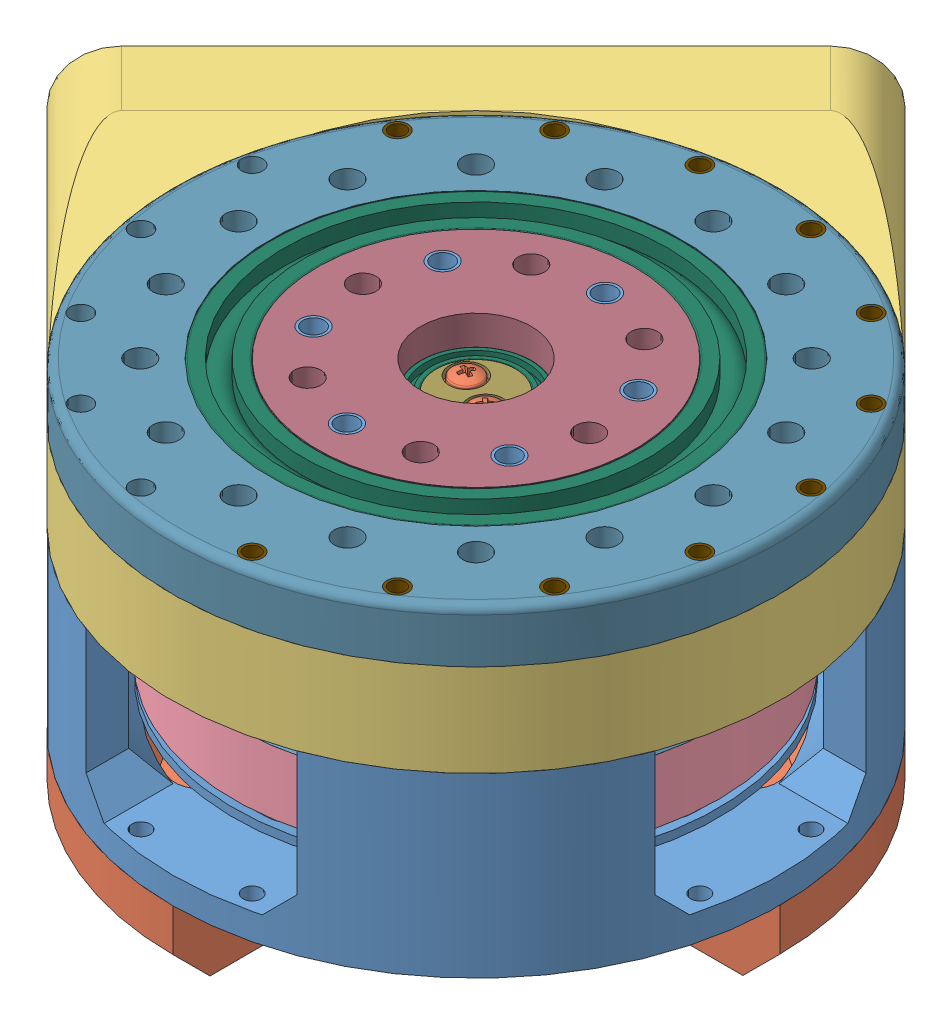
SolidWorks assembly Cycloidal_v2, configuration Default. Lengths in mm. (continued)
Components (placement in the parent): (continued)
- hex nut style 1 gradeab_iso-1: hex nut style 1 gradeab_iso [ISO - 4032 - M3 - W - N] at (47.267 33.7573 119.5643) x (1 0 0) z (0 -1 0) size (5.5 6.35 2.4)
- Cycloidal_Discs_8308-1: Cycloidal_Discs_8308 [Default] at (41.9439 42.227 18.4807) x (0.879085 0 0.476665) z (-0.476665 0 0.879085) size (79.25 5 79.73)
  - Cycloidal_Discs-1: Cycloidal_Discs [Default] at (38.3081 39.5303 58.0959) size (79.25 5 79.73)
  - radial ball bearing_68_iso-1: radial ball bearing_68_iso [ISO 15 RBB - 274 - 14,SI,NC,14_68] at (18.3896 43.2803 46.5959) x (0 1 0) z (0 0 1) size (2.5 7 7)
  - radial ball bearing_68_iso-2: radial ball bearing_68_iso [ISO 15 RBB - 274 - 14,SI,NC,14_68] at (38.3081 43.2803 81.0959) x (0 1 0) z (0 0 1) size (2.5 7 7)
  - radial ball bearing_68_iso-3: radial ball bearing_68_iso [ISO 15 RBB - 274 - 14,SI,NC,14_68] at (18.3896 43.2803 69.5959) x (0 1 0) z (0 0 1) size (2.5 7 7)
  - radial ball bearing_68_iso-4: radial ball bearing_68_iso [ISO 15 RBB - 274 - 14,SI,NC,14_68] at (38.3081 43.2803 35.0959) x (0 1 0) z (0 0 1) size (2.5 7 7)
  - radial ball bearing_68_iso-5: radial ball bearing_68_iso [ISO 15 RBB - 274 - 14,SI,NC,14_68] at (58.2267 43.2803 69.5959) x (0 1 0) z (0 0 1) size (2.5 7 7)
  - radial ball bearing_68_iso-6: radial ball bearing_68_iso [ISO 15 RBB - 274 - 14,SI,NC,14_68] at (58.2267 43.2803 46.5959) x (0 1 0) z (0 0 1) size (2.5 7 7)
- Cycloidal_Discs_8308-2: Cycloidal_Discs_8308 [Default] at (110.2095 37.227 62.2693) x (-0.1644 0 0.986394) z (-0.986394 0 -0.1644) size (79.25 5 79.73)
  - Cycloidal_Discs-1: Cycloidal_Discs [Default] at (38.3081 39.5303 58.0959) size (79.25 5 79.73)
  - radial ball bearing_68_iso-1: radial ball bearing_68_iso [ISO 15 RBB - 274 - 14,SI,NC,14_68] at (18.3896 43.2803 46.5959) x (0 1 0) z (0 0 1) size (2.5 7 7)
  - radial ball bearing_68_iso-2: radial ball bearing_68_iso [ISO 15 RBB - 274 - 14,SI,NC,14_68] at (38.3081 43.2803 81.0959) x (0 1 0) z (0 0 1) size (2.5 7 7)
  - radial ball bearing_68_iso-3: radial ball bearing_68_iso [ISO 15 RBB - 274 - 14,SI,NC,14_68] at (18.3896 43.2803 69.5959) x (0 1 0) z (0 0 1) size (2.5 7 7)
  - radial ball bearing_68_iso-4: radial ball bearing_68_iso [ISO 15 RBB - 274 - 14,SI,NC,14_68] at (38.3081 43.2803 35.0959) x (0 1 0) z (0 0 1) size (2.5 7 7)
  - radial ball bearing_68_iso-5: radial ball bearing_68_iso [ISO 15 RBB - 274 - 14,SI,NC,14_68] at (58.2267 43.2803 69.5959) x (0 1 0) z (0 0 1) size (2.5 7 7)
  - radial ball bearing_68_iso-6: radial ball bearing_68_iso [ISO 15 RBB - 274 - 14,SI,NC,14_68] at (58.2267 43.2803 46.5959) x (0 1 0) z (0 0 1) size (2.5 7 7)
- m6-1: m6 [Default] at (24.3171 92.633 87.6415) x (0 0 -1) z (-1 0 0) size (6 16 6)
- Motor_Cover_v2-2: Motor_Cover_v2 [Default] at (47.267 36.1573 89.1587) x (-1 0 0) z (0 0 -1) size (115 33.6 115)
- driver_cover-1: driver_cover [Default] at (47.267 36.1573 89.1587) x (-0.70834 0 -0.705872) z (-0.705872 0 0.70834) size (81.32 15 115)
- Base_plate_2 _new-1: Base_plate_2 _new [Default] at (47.267 69.6573 89.1587) x (-0.707107 0 0.707107) z (-0.707107 0 -0.707107) size (115 87.5 130)
Mates (geometry in assembly coordinates):
- Coincident1: coincident anti-aligned: plane of motor-X83008S.stp-1/outrunner.stp-1 through (62.4642 69.7573 58.1862) normal (0 1 0); plane of Base_Plate-1 through (47.267 69.7573 89.1587) normal (0 -1 0)
- Concentric1: concentric anti-aligned: line of motor-X83008S.stp-1/outrunner.stp-1 through (54.0947 64.2573 75.2435) axis (0 1 0); cylinder of Base_Plate-1 through (54.0947 76.7573 75.2435) axis (0 -1 0) radius 1.5
- Concentric2: concentric anti-aligned: cylinder of motor-X83008S.stp-1/shaft.stp-1 through (47.267 69.7573 89.1587) axis (0 1 0) radius 1.5; line of Base_Plate-1 through (47.267 76.7573 89.1587) axis (0 -1 0)
- Coincident2: coincident anti-aligned: plane of Base_Plate-1 through (47.267 76.7573 89.1587) normal (0 1 0); plane of Eccentric_Shaft-1/Eccentric_Shaft_bot-1 through (46.6062 76.7573 90.5053) normal (0 -1 0)
- Concentric75: concentric anti-aligned: cylinder of Output_Shaft-1 through (47.267 97.2573 89.1587) axis (0 -1 0) radius 30; cylinder of radial ball bearing_68_iso-39 through (47.267 71.6198 89.1587) axis (0 1 0) radius 30
- Concentric76: concentric anti-aligned: cylinder of Cover-1 through (47.267 97.2573 89.1587) axis (0 -1 0) radius 39; cylinder of radial ball bearing_68_iso-39 through (47.267 71.6198 89.1587) axis (0 1 0) radius 39
- Coincident104: coincident aligned: plane of Cover-1 through (47.267 97.2573 89.1587) normal (0 1 0); plane of radial ball bearing_68_iso-39 through (8.567 97.2573 89.1587) normal (0 1 0)
- Coincident105: coincident aligned: plane of Output_Shaft-1 through (47.267 97.2573 89.1587) normal (0 1 0); plane of Cover-1 through (47.267 97.2573 89.1587) normal (0 1 0)
- Concentric78: concentric anti-aligned: cylinder of Base_Plate-1 through (47.267 76.7573 89.1587) axis (0 -1 0) radius 20; cylinder of radial ball bearing_68_iso-40 through (47.267 52.6198 89.1587) axis (0 1 0) radius 20
- Concentric84: concentric aligned: cylinder of Cover-1 through (15.4472 87.2573 57.3389) axis (0 1 0) radius 2.5; cylinder of m13_bearing-1/m6-1 through (15.4472 86.8573 57.3389) axis (0 1 0) radius 2
- Concentric85: concentric aligned: cylinder of Cover-1 through (47.267 87.2573 134.1587) axis (0 1 0) radius 2.5; cylinder of m13_bearing-11/m6-1 through (47.267 86.8573 134.1587) axis (0 1 0) radius 2
- Concentric86: concentric aligned: cylinder of Cover-1 through (64.4877 87.2573 130.7332) axis (0 1 0) radius 2.5; cylinder of m13_bearing-2/m6-1 through (64.4877 86.8573 130.7332) axis (0 1 0) radius 2
- Concentric87: concentric aligned: cylinder of Cover-1 through (79.0868 87.2573 120.9785) axis (0 1 0) radius 2.5; cylinder of m13_bearing-12/m6-1 through (79.0868 86.8573 120.9785) axis (0 1 0) radius 2
- Concentric88: concentric aligned: cylinder of Cover-1 through (88.8416 87.2573 106.3794) axis (0 1 0) radius 2.5; cylinder of m13_bearing-5/m6-1 through (88.8416 86.8573 106.3794) axis (0 1 0) radius 2
- Concentric89: concentric aligned: cylinder of Cover-1 through (92.267 87.2573 89.1587) axis (0 1 0) radius 2.5; cylinder of m13_bearing-4/m6-1 through (92.267 86.8573 89.1587) axis (0 1 0) radius 2
- Concentric90: concentric aligned: cylinder of Cover-1 through (30.0462 87.2573 47.5841) axis (0 1 0) radius 2.5; cylinder of m13_bearing-6/m6-1 through (30.0462 86.8573 47.5841) axis (0 1 0) radius 2
- Concentric91: concentric aligned: cylinder of Cover-1 through (47.267 87.2573 44.1587) axis (0 1 0) radius 2.5; cylinder of m13_bearing-3/m6-1 through (47.267 86.8573 44.1587) axis (0 1 0) radius 2
- Concentric92: concentric aligned: cylinder of Cover-1 through (64.4877 87.2573 47.5841) axis (0 1 0) radius 2.5; cylinder of m13_bearing-7/m6-1 through (64.4877 86.8573 47.5841) axis (0 1 0) radius 2
- Concentric93: concentric aligned: cylinder of Cover-1 through (79.0868 87.2573 57.3389) axis (0 1 0) radius 2.5; cylinder of m13_bearing-8/m6-1 through (79.0868 86.8573 57.3389) axis (0 1 0) radius 2
- Concentric94: concentric aligned: cylinder of Cover-1 through (88.8416 87.2573 71.9379) axis (0 1 0) radius 2.5; cylinder of m13_bearing-9/m6-1 through (88.8416 86.8573 71.9379) axis (0 1 0) radius 2
- Concentric118: concentric anti-aligned: cylinder of Output_Shaft-1 through (60.0558 97.2573 70.042) axis (0 -1 0) radius 2.5; cylinder of M4x6x5.5_brass_insert-1 through (60.0558 86.633 70.042) axis (0 1 0) radius 2
- Concentric1211: concentric aligned: cylinder of Cover-1 through (2.3676 97.2573 59.1579) axis (0 -1 0) radius 2; cylinder of M3x4x4.2_brass_insert-2 through (2.3676 92.3553 59.1579) axis (0 -1 0) radius 1.5
- Concentric1221: concentric aligned: cylinder of Cover-1 through (17.2662 97.2573 44.2593) axis (0 -1 0) radius 2; cylinder of M3x4x4.2_brass_insert-3 through (17.2662 92.3553 44.2593) axis (0 -1 0) radius 1.5
- Concentric1251: concentric aligned: cylinder of Cover-1 through (77.2678 97.2573 44.2593) axis (0 -1 0) radius 2; cylinder of M3x4x4.2_brass_insert-6 through (77.2678 92.3553 44.2593) axis (0 -1 0) radius 1.8
- Concentric1271: concentric anti-aligned: cylinder of Cover-1 through (100.2294 97.2573 78.6238) axis (0 -1 0) radius 2; cylinder of M3x4x4.2_brass_insert-8 through (100.2294 98.1594 78.6238) axis (0 1 0) radius 1.8
- Concentric1331: concentric aligned: cylinder of Cover-1 through (36.7321 97.2573 36.1963) axis (0 -1 0) radius 2; cylinder of M3x4x4.2_brass_insert-14 through (36.7321 92.3553 36.1963) axis (0 -1 0) radius 1.8
- Concentric1341: concentric anti-aligned: cylinder of Cover-1 through (57.8019 97.2573 36.1963) axis (0 -1 0) radius 2; cylinder of M3x4x4.2_brass_insert-15 through (57.8019 98.1594 36.1963) axis (0 1 0) radius 2
- Concentric1351: concentric aligned: cylinder of Cover-1 through (92.1663 97.2573 59.1579) axis (0 -1 0) radius 2; cylinder of M3x4x4.2_brass_insert-16 through (92.1663 92.3553 59.1579) axis (0 -1 0) radius 2
- Concentric1361: concentric aligned: cylinder of Cover-1 through (100.2294 97.2573 99.6935) axis (0 -1 0) radius 2; cylinder of M3x4x4.2_brass_insert-17 through (100.2294 92.3553 99.6935) axis (0 -1 0) radius 2
- Concentric1381: concentric aligned: cylinder of Cover-1 through (92.1663 97.2573 119.1595) axis (0 -1 0) radius 2; cylinder of M3x4x4.2_brass_insert-19 through (92.1663 92.3553 119.1595) axis (0 -1 0) radius 2
- Concentric1391: concentric aligned: cylinder of Cover-1 through (77.2678 97.2573 134.058) axis (0 -1 0) radius 2; cylinder of M3x4x4.2_brass_insert-20 through (77.2678 92.3553 134.058) axis (0 -1 0) radius 1.5
- Concentric1401: concentric aligned: cylinder of Cover-1 through (57.8019 97.2573 142.1211) axis (0 -1 0) radius 2; cylinder of M3x4x4.2_brass_insert-21 through (57.8019 92.3553 142.1211) axis (0 -1 0) radius 1.5
- Concentric14021: concentric aligned: cylinder of Output_Shaft-1 through (57.4281 97.2573 109.7924) axis (0 -1 0) radius 2.5; cylinder of M4x6x5.5_brass_insert-4 through (57.4281 80.689 109.7924) axis (0 -1 0) radius 2.5
- Concentric14031: concentric aligned: cylinder of Output_Shaft-1 through (34.4782 97.2573 108.2753) axis (0 -1 0) radius 2.5; cylinder of M4x6x5.5_brass_insert-5 through (34.4782 80.689 108.2753) axis (0 -1 0) radius 2.5
- Concentric14041: concentric aligned: cylinder of Output_Shaft-1 through (24.3171 97.2573 87.6415) axis (0 -1 0) radius 2.5; cylinder of M4x6x5.5_brass_insert-6 through (24.3171 80.689 87.6415) axis (0 -1 0) radius 2.5
- Concentric14051: concentric aligned: cylinder of Output_Shaft-1 through (37.1059 97.2573 68.5249) axis (0 -1 0) radius 2.5; cylinder of M4x6x5.5_brass_insert-7 through (37.1059 80.689 68.5249) axis (0 -1 0) radius 2.5
- Concentric14061: concentric aligned: cylinder of Output_Shaft-1 through (67.9008 97.2573 78.9976) axis (0 -1 0) radius 2.5; cylinder of M4x6x5.5_brass_insert-8 through (67.9008 85.3133 78.9976) axis (0 -1 0) radius 2.5
- Concentric14071: concentric aligned: cylinder of Output_Shaft-1 through (48.7841 97.2573 66.2088) axis (0 -1 0) radius 2.5; cylinder of M4x6x5.5_brass_insert-9 through (48.7841 85.3133 66.2088) axis (0 -1 0) radius 2.5
- Concentric14081: concentric aligned: cylinder of Output_Shaft-1 through (28.1503 97.2573 76.3698) axis (0 -1 0) radius 2.5; cylinder of M4x6x5.5_brass_insert-10 through (28.1503 85.3133 76.3698) axis (0 -1 0) radius 2.5
- Concentric14091: concentric aligned: cylinder of Output_Shaft-1 through (26.6332 97.2573 99.3197) axis (0 -1 0) radius 2.5; cylinder of M4x6x5.5_brass_insert-11 through (26.6332 85.3133 99.3197) axis (0 -1 0) radius 2.5
- Concentric14111: concentric aligned: cylinder of Output_Shaft-1 through (45.7499 97.2573 112.1086) axis (0 -1 0) radius 2.5; cylinder of M4x6x5.5_brass_insert-13 through (45.7499 85.3133 112.1086) axis (0 -1 0) radius 2.5
- Concentric14121: concentric aligned: cylinder of Output_Shaft-1 through (66.3836 97.2573 101.9475) axis (0 -1 0) radius 2.5; cylinder of M4x6x5.5_brass_insert-14 through (66.3836 85.3133 101.9475) axis (0 -1 0) radius 2.5
- Concentric14131: concentric aligned: cylinder of Output_Shaft-1 through (70.2169 97.2573 90.6758) axis (0 -1 0) radius 2.5; cylinder of M4x6x5.5_brass_insert-15 through (70.2169 80.689 90.6758) axis (0 -1 0) radius 2.5
- Coincident1435: coincident aligned: plane of M4x6x5.5_brass_insert-1 through (58.1912 92.633 71.7074) normal (0 1 0); plane of M4x6x5.5_brass_insert-15 through (70.2169 92.633 90.6758) normal (0 1 0)
- Coincident1436: coincident aligned: plane of M4x6x5.5_brass_insert-1 through (58.1912 92.633 71.7074) normal (0 1 0); plane of M4x6x5.5_brass_insert-4 through (57.4281 92.633 109.7924) normal (0 1 0)
- Coincident1437: coincident aligned: plane of M4x6x5.5_brass_insert-1 through (58.1912 92.633 71.7074) normal (0 1 0); plane of M4x6x5.5_brass_insert-5 through (34.4782 92.633 108.2753) normal (0 1 0)
- Coincident1438: coincident aligned: plane of M4x6x5.5_brass_insert-1 through (58.1912 92.633 71.7074) normal (0 1 0); plane of M4x6x5.5_brass_insert-6 through (24.3171 92.633 87.6415) normal (0 1 0)
- Coincident1439: coincident aligned: plane of M4x6x5.5_brass_insert-1 through (58.1912 92.633 71.7074) normal (0 1 0); plane of M4x6x5.5_brass_insert-7 through (37.1059 92.633 68.5249) normal (0 1 0)
- Coincident1440: coincident aligned: plane of Output_Shaft-1 through (47.267 97.2573 89.1587) normal (0 1 0); plane of M4x6x5.5_brass_insert-9 through (48.7841 97.2573 66.2088) normal (0 1 0)
- Coincident1441: coincident aligned: plane of Output_Shaft-1 through (47.267 97.2573 89.1587) normal (0 1 0); plane of M4x6x5.5_brass_insert-8 through (67.9008 97.2573 78.9976) normal (0 1 0)
- Coincident1442: coincident aligned: plane of Output_Shaft-1 through (47.267 97.2573 89.1587) normal (0 1 0); plane of M4x6x5.5_brass_insert-14 through (66.3836 97.2573 101.9475) normal (0 1 0)
- Coincident1443: coincident aligned: plane of Output_Shaft-1 through (47.267 97.2573 89.1587) normal (0 1 0); plane of M4x6x5.5_brass_insert-13 through (45.7499 97.2573 112.1086) normal (0 1 0)
- Coincident1444: coincident aligned: plane of Output_Shaft-1 through (47.267 97.2573 89.1587) normal (0 1 0); plane of M4x6x5.5_brass_insert-11 through (26.6332 97.2573 99.3197) normal (0 1 0)
- Coincident1445: coincident aligned: plane of Output_Shaft-1 through (47.267 97.2573 89.1587) normal (0 1 0); plane of M4x6x5.5_brass_insert-10 through (28.1503 97.2573 76.3698) normal (0 1 0)
- Concentric14151: concentric aligned: cylinder of m13_bearing-2/m6-1 through (64.4877 86.8573 130.7332) axis (0 1 0) radius 2; cylinder of M4x6x5.5_brass_insert-20 through (64.4877 86.8573 130.7332) axis (0 1 0) radius 2
- Concentric14161: concentric aligned: cylinder of m13_bearing-11/m6-1 through (47.267 86.8573 134.1587) axis (0 1 0) radius 2; cylinder of M4x6x5.5_brass_insert-21 through (47.267 86.8573 134.1587) axis (0 1 0) radius 2
- Concentric14171: concentric aligned: cylinder of m13_bearing-1/m6-1 through (15.4472 86.8573 57.3389) axis (0 1 0) radius 2; cylinder of M4x6x5.5_brass_insert-22 through (15.4472 86.8573 57.3389) axis (0 1 0) radius 2
- Concentric14181: concentric aligned: cylinder of m13_bearing-6/m6-1 through (30.0462 86.8573 47.5841) axis (0 1 0) radius 2; cylinder of M4x6x5.5_brass_insert-23 through (30.0462 86.8573 47.5841) axis (0 1 0) radius 2
- Concentric14191: concentric aligned: cylinder of m13_bearing-12/m6-1 through (79.0868 86.8573 120.9785) axis (0 1 0) radius 2; cylinder of M4x6x5.5_brass_insert-24 through (79.0868 98.8014 120.9785) axis (0 1 0) radius 2.3
- Concentric14201: concentric aligned: cylinder of m13_bearing-5/m6-1 through (88.8416 86.8573 106.3794) axis (0 1 0) radius 2; cylinder of M4x6x5.5_brass_insert-25 through (88.8416 86.8573 106.3794) axis (0 1 0) radius 2
- Concentric14211: concentric aligned: cylinder of m13_bearing-4/m6-1 through (92.267 86.8573 89.1587) axis (0 1 0) radius 2; cylinder of M4x6x5.5_brass_insert-26 through (92.267 86.8573 89.1587) axis (0 1 0) radius 2
- Concentric14221: concentric aligned: cylinder of m13_bearing-9/m6-1 through (88.8416 86.8573 71.9379) axis (0 1 0) radius 2; cylinder of M4x6x5.5_brass_insert-27 through (88.8416 86.8573 71.9379) axis (0 1 0) radius 2
- Concentric14241: concentric aligned: cylinder of m13_bearing-7/m6-1 through (64.4877 86.8573 47.5841) axis (0 1 0) radius 2; cylinder of M4x6x5.5_brass_insert-29 through (64.4877 86.8573 47.5841) axis (0 1 0) radius 2
- Concentric14251: concentric aligned: cylinder of m13_bearing-3/m6-1 through (47.267 86.8573 44.1587) axis (0 1 0) radius 2; cylinder of M4x6x5.5_brass_insert-31 through (47.267 86.8573 44.1587) axis (0 1 0) radius 2
- Coincident1447: coincident anti-aligned: plane of m13_bearing-2/m6-1 through (64.4877 86.8573 130.7332) normal (0 1 0); plane of M4x6x5.5_brass_insert-20 through (64.4877 86.8573 130.7332) normal (0 -1 0)
- Coincident1458: coincident aligned: plane of M4x6x5.5_brass_insert-20 through (62.6232 92.8573 132.3986) normal (0 1 0); plane of M4x6x5.5_brass_insert-21 through (45.4024 92.8573 135.824) normal (0 1 0)
- Coincident1459: coincident aligned: plane of M4x6x5.5_brass_insert-20 through (62.6232 92.8573 132.3986) normal (0 1 0); plane of M4x6x5.5_brass_insert-22 through (17.0054 92.8573 59.2938) normal (0 1 0)
- Coincident1460: coincident aligned: plane of M4x6x5.5_brass_insert-20 through (62.6232 92.8573 132.3986) normal (0 1 0); plane of M4x6x5.5_brass_insert-23 through (31.6045 92.8573 49.5391) normal (0 1 0)
- Coincident1461: coincident aligned: plane of M4x6x5.5_brass_insert-20 through (62.6232 92.8573 132.3986) normal (0 1 0); plane of M4x6x5.5_brass_insert-31 through (46.7161 92.8573 46.5972) normal (0 1 0)
- Coincident1462: coincident aligned: plane of M4x6x5.5_brass_insert-20 through (62.6232 92.8573 132.3986) normal (0 1 0); plane of M4x6x5.5_brass_insert-29 through (64.1304 92.8573 50.0584) normal (0 1 0)
- Coincident1463: coincident aligned: plane of M4x6x5.5_brass_insert-20 through (62.6232 92.8573 132.3986) normal (0 1 0); plane of M4x6x5.5_brass_insert-28 through (79.0868 92.8573 57.3389) normal (0 1 0)
- Coincident1464: coincident aligned: plane of M4x6x5.5_brass_insert-20 through (62.6232 92.8573 132.3986) normal (0 1 0); plane of M4x6x5.5_brass_insert-27 through (86.977 92.8573 73.6032) normal (0 1 0)
- Coincident1465: coincident aligned: plane of M4x6x5.5_brass_insert-20 through (62.6232 92.8573 132.3986) normal (0 1 0); plane of M4x6x5.5_brass_insert-26 through (90.4024 92.8573 90.824) normal (0 1 0)
- Coincident1466: coincident aligned: plane of M4x6x5.5_brass_insert-20 through (62.6232 92.8573 132.3986) normal (0 1 0); plane of M4x6x5.5_brass_insert-25 through (86.977 92.8573 108.0448) normal (0 1 0)
- Coincident1467: coincident aligned: plane of M4x6x5.5_brass_insert-20 through (62.6232 92.8573 132.3986) normal (0 1 0); plane of M4x6x5.5_brass_insert-24 through (80.4417 92.8573 123.0795) normal (0 1 0)
- Concentric1426: concentric aligned: cylinder of pan cross head_am-1 through (50.858 118.0573 90.9207) axis (0 1 0) radius 1.5; line of Eccentric_Shaft-1/Eccentric_Shaft_top-1 through (50.858 90.2573 90.9207) axis (0 1 0)
- Coincident1468: coincident anti-aligned: plane of Eccentric_Shaft-1/Eccentric_Shaft_top-1 through (43.676 90.2573 87.3967) normal (0 1 0); plane of pan cross head_am-1 through (51.8522 90.2573 89.7974) normal (0 -1 0)
- Concentric14281: concentric aligned: cylinder of pan cross head_am-3 through (43.676 118.0573 87.3967) axis (0 1 0) radius 2.8; cylinder of Eccentric_Shaft-1/Eccentric_Shaft_top-1 through (43.676 86.7573 87.3967) axis (0 1 0) radius 1.5
- Coincident14701: coincident anti-aligned: plane of Eccentric_Shaft-1/Eccentric_Shaft_top-1 through (50.858 90.2573 90.9207) normal (0 1 0); plane of pan cross head_am-3 through (44.1864 90.2573 85.9862) normal (0 -1 0)
- Concentric1437: concentric anti-aligned: cylinder of Base_Plate-1 through (50.858 76.7573 90.9207) axis (0 -1 0) radius 2; cylinder of M3x4x4.2_brass_insert-22 through (50.858 74.6594 90.9207) axis (0 1 0) radius 1.5
- Coincident1479: coincident aligned: plane of Base_Plate-1 through (47.267 69.7573 89.1587) normal (0 -1 0); plane of M3x4x4.2_brass_insert-22 through (52.3349 69.7573 90.6583) normal (0 -1 0)
- Concentric1438: concentric anti-aligned: cylinder of Base_Plate-1 through (43.676 76.7573 87.3967) axis (0 -1 0) radius 2; cylinder of M3x4x4.2_brass_insert-23 through (43.676 74.6594 87.3967) axis (0 1 0) radius 1.5
- Coincident1480: coincident aligned: plane of Base_Plate-1 through (47.267 69.7573 89.1587) normal (0 -1 0); plane of M3x4x4.2_brass_insert-23 through (45.1529 69.7573 87.1345) normal (0 -1 0)
- Concentric1439: concentric anti-aligned: cylinder of Base_Plate-1 through (33.3518 76.7573 82.3309) axis (0 -1 0) radius 1.5; cylinder of pan cross head_am-4 through (33.3518 103.0573 82.3309) axis (0 1 0) radius 1.5
- Coincident1481: coincident anti-aligned: plane of Base_Plate-1 through (33.3518 75.2573 82.3309) normal (0 1 0); plane of pan cross head_am-4 through (34.8518 75.2573 82.3309) normal (0 -1 0)
- Concentric14401: concentric anti-aligned: cylinder of Base_Plate-1 through (61.1822 76.7573 95.9864) axis (0 -1 0) radius 1.5; cylinder of pan cross head_am-5 through (61.1822 103.0573 95.9864) axis (0 1 0) radius 2.8
- Coincident14821: coincident anti-aligned: plane of Base_Plate-1 through (61.1822 75.2573 95.9864) normal (0 1 0); plane of pan cross head_am-5 through (62.6822 75.2573 95.9864) normal (0 -1 0)
- GearMate1: gear = 10 : 1 mm: cylinder of Eccentric_Shaft-1/Eccentric_Shaft_top-1 through (47.267 91.7573 89.1587) axis (0 -1 0) radius 7.5; cylinder of Output_Shaft-1 through (47.267 97.2573 89.1587) axis (0 -1 0) radius 10.5
- Concentric1445021: concentric anti-aligned: cylinder of Base_Plate-1 through (40.4392 76.7573 103.0738) axis (0 -1 0) radius 1.5; cylinder of pan cross head_am-6 through (40.4392 103.0573 103.0738) axis (0 1 0) radius 2.8
- Coincident1486621: coincident anti-aligned: plane of Base_Plate-1 through (40.4392 75.2573 103.0738) normal (0 1 0); plane of pan cross head_am-6 through (41.9392 75.2573 103.0738) normal (0 -1 0)
- Concentric1445031: concentric anti-aligned: cylinder of Base_Plate-1 through (54.0947 76.7573 75.2435) axis (0 -1 0) radius 1.5; cylinder of pan cross head_am-7 through (54.0947 103.0573 75.2435) axis (0 1 0) radius 2.8
- Coincident1486631: coincident anti-aligned: plane of Base_Plate-1 through (54.0947 75.2573 75.2435) normal (0 1 0); plane of pan cross head_am-7 through (55.5947 75.2573 75.2435) normal (0 -1 0)
- Coincident1486632: coincident anti-aligned: plane of Cover-1 through (88.8416 86.8573 71.9379) normal (0 -1 0); plane of m13_bearing-9/radial ball bearing_68_iso-2 through (91.6245 86.8573 68.9955) normal (0 1 0)
- Coincident1486633: coincident anti-aligned: plane of Cover-1 through (88.8416 86.8573 71.9379) normal (0 -1 0); plane of m13_bearing-8/radial ball bearing_68_iso-2 through (78.4447 86.8573 53.3401) normal (0 1 0)
- Coincident1486634: coincident anti-aligned: plane of Cover-1 through (88.8416 86.8573 71.9379) normal (0 -1 0); plane of m13_bearing-7/radial ball bearing_68_iso-2 through (66.6983 86.8573 44.1906) normal (0 1 0)
- Coincident1486635: coincident anti-aligned: plane of Cover-1 through (88.8416 86.8573 71.9379) normal (0 -1 0); plane of m13_bearing-3/radial ball bearing_68_iso-2 through (47.4539 86.8573 40.113) normal (0 1 0)
- Coincident1486636: coincident anti-aligned: plane of Cover-1 through (88.8416 86.8573 71.9379) normal (0 -1 0); plane of m13_bearing-4/radial ball bearing_68_iso-2 through (92.1768 86.8573 85.1097) normal (0 1 0)
- Coincident1486637: coincident anti-aligned: plane of Cover-1 through (88.8416 86.8573 71.9379) normal (0 -1 0); plane of m13_bearing-5/radial ball bearing_68_iso-2 through (88.6021 86.8573 102.3365) normal (0 1 0)
- Coincident1486638: coincident anti-aligned: plane of Cover-1 through (88.8416 86.8573 71.9379) normal (0 -1 0); plane of m13_bearing-12/radial ball bearing_68_iso-2 through (78.3409 86.8573 116.9978) normal (0 1 0)
- Coincident1486639: coincident anti-aligned: plane of Cover-1 through (88.8416 86.8573 71.9379) normal (0 -1 0); plane of m13_bearing-11/radial ball bearing_68_iso-2 through (44.9443 86.8573 130.8409) normal (0 1 0)
- Coincident1486640: coincident anti-aligned: plane of Cover-1 through (88.8416 86.8573 71.9379) normal (0 -1 0); plane of m13_bearing-2/radial ball bearing_68_iso-2 through (64.0006 86.8573 126.7126) normal (0 1 0)
- Coincident1486643: coincident anti-aligned: plane of Cover-1 through (30.0462 86.8573 47.5841) normal (0 -1 0); plane of m13_bearing-6/radial ball bearing_68_iso-2 through (28.2174 86.8573 43.9705) normal (0 1 0)
- Coincident1486644: coincident anti-aligned: plane of Cover-1 through (15.4472 86.8573 57.3389) normal (0 -1 0); plane of m13_bearing-1/radial ball bearing_68_iso-2 through (12.4643 86.8573 54.5994) normal (0 1 0)
- Concentric1445035: concentric anti-aligned: cylinder of Eccentric_Shaft-1/Eccentric_Shaft_bot-1 through (46.6062 81.7573 90.5053) axis (0 -1 0) radius 7.5; cylinder of radial ball bearing_68_iso-46 through (46.6062 59.1198 90.5053) axis (0 1 0) radius 7.5
- Coincident1486648: coincident aligned: plane of Eccentric_Shaft-1/Eccentric_Shaft_bot-1 through (46.6062 81.7573 90.5053) normal (0 1 0); plane of radial ball bearing_68_iso-46 through (38.9062 81.7573 90.5067) normal (0 1 0)
- Concentric1445036: concentric anti-aligned: cylinder of Eccentric_Shaft-1/Eccentric_Shaft_bot-2 through (47.9277 86.7573 87.812) axis (0 -1 0) radius 7.5; cylinder of radial ball bearing_68_iso-44 through (47.9277 64.1198 87.812) axis (0 1 0) radius 7.5
- Coincident1486649: coincident aligned: plane of Eccentric_Shaft-1/Eccentric_Shaft_bot-2 through (47.9277 82.7573 87.812) normal (0 1 0); circle of radial ball bearing_68_iso-44
- Concentric1445037: concentric anti-aligned: cylinder of Eccentric_Shaft-1/Eccentric_Shaft_top-1 through (47.267 91.7573 89.1587) axis (0 -1 0) radius 7.5; cylinder of radial ball bearing_68_iso-45 through (47.267 69.1198 89.1587) axis (0 1 0) radius 7.5
- Concentric1445038: concentric anti-aligned: cylinder of Base_Plate-1 through (47.267 76.7573 89.1587) axis (0 -1 0) radius 20; cylinder of radial ball bearing_68_iso-40 through (47.267 52.6198 89.1587) axis (0 1 0) radius 20
- Coincident1486655: coincident anti-aligned: plane of Eccentric_Shaft-1/Eccentric_Shaft_top-1 through (47.267 87.7573 89.1587) normal (0 1 0); plane of radial ball bearing_68_iso-45 through (47.5372 87.7573 97.5543) normal (0 -1 0)
- Concentric1445042: concentric anti-aligned: cylinder of Base_Plate-1 through (43.676 76.7573 87.3967) axis (0 -1 0) radius 2; cylinder of Eccentric_Shaft-1/Eccentric_Shaft_bot-1 through (43.676 76.7573 87.3967) axis (0 1 0) radius 1.5
- Concentric1445043: concentric aligned: cylinder of Eccentric_Shaft-1/Eccentric_Shaft_bot-1 through (50.858 76.7573 90.9207) axis (0 1 0) radius 1.5; cylinder of M3x4x4.2_brass_insert-22 through (50.858 74.6594 90.9207) axis (0 1 0) radius 1.5
- Coincident1486660: coincident aligned: plane of Cover-1 through (5.6924 86.8573 71.9379) normal (0 -1 0); circle of m13_bearing-31/radial ball bearing_68_iso-2
- Coincident1486661: coincident aligned: plane of Cover-1 through (5.6924 86.8573 71.9379) normal (0 -1 0); circle of m13_bearing-32/radial ball bearing_68_iso-2
- Coincident1486662: coincident aligned: plane of Cover-1 through (5.6924 86.8573 71.9379) normal (0 -1 0); circle of m13_bearing-36/radial ball bearing_68_iso-2
- Coincident1486663: coincident aligned: plane of Cover-1 through (5.6924 86.8573 71.9379) normal (0 -1 0); circle of m13_bearing-35/radial ball bearing_68_iso-2
- Coincident1486664: coincident aligned: plane of Cover-1 through (5.6924 86.8573 71.9379) normal (0 -1 0); circle of m13_bearing-34/radial ball bearing_68_iso-2
- Concentric1445052: concentric aligned: circle of m13_bearing-31/m6-1; cylinder of M4x6x5.5_brass_insert-47 through (5.6924 92.8573 71.9379) axis (0 -1 0) radius 2
- Concentric14450531: concentric aligned: line of Cover-1 through (5.6924 86.8573 106.3794) axis (0 1 0); cylinder of M4x6x5.5_brass_insert-49 through (5.6924 87.0073 106.3794) axis (0 1 0) radius 2
- Concentric14450541: concentric aligned: line of Cover-1 through (15.4472 86.8573 120.9785) axis (0 1 0); cylinder of M4x6x5.5_brass_insert-50 through (15.4472 86.8573 120.9785) axis (0 1 0) radius 2
- Concentric1445056: concentric aligned: circle of m13_bearing-32/m6-1; cylinder of M4x6x5.5_brass_insert-48 through (2.267 92.8573 89.1587) axis (0 -1 0) radius 2
- Coincident1486681: coincident anti-aligned: plane of m13_bearing-1/m6-1 through (15.4472 92.8573 57.3389) normal (0 1 0); circle of M4x6x5.5_brass_insert-47
- Concentric1445063: concentric aligned: cylinder of m13_bearing-34/m6-1 through (30.0462 87.0073 130.7332) axis (0 1 0) radius 2; cylinder of M4x6x5.5_brass_insert-51 through (30.0462 87.0073 130.7332) axis (0 1 0) radius 2
- Coincident1486686: coincident aligned: plane of m13_bearing-36/m6-1 through (5.6924 93.0073 106.3794) normal (0 1 0); circle of M4x6x5.5_brass_insert-49
- Coincident1486687: coincident anti-aligned: plane of m13_bearing-32/m6-1 through (2.267 92.8573 89.1587) normal (0 1 0); circle of M4x6x5.5_brass_insert-48
- Coincident1486688: coincident aligned: plane of m13_bearing-35/m6-1 through (15.4472 92.8573 120.9785) normal (0 1 0); circle of M4x6x5.5_brass_insert-50
- Coincident1486690: coincident aligned: plane of m13_bearing-34/m6-1 through (30.0462 93.0073 130.7332) normal (0 1 0); circle of M4x6x5.5_brass_insert-51
- Coincident1486692: coincident anti-aligned: plane of foc-motor-controller.step-1/foc-motor-controller_PCB.step-1 through (47.267 33.7573 89.1587) normal (0 1 0); plane of hex nut style 1 gradeab_iso-1 through (47.267 33.7573 122.7397) normal (0 -1 0)
- Concentric14450545: concentric anti-aligned: cylinder of radial ball bearing_68_iso-46 through (46.6062 59.1198 90.5053) axis (0 1 0) radius 10.5; cylinder of Cycloidal_Discs_8308-2/Cycloidal_Discs-1 through (46.6062 81.7573 90.5053) axis (0 -1 0) radius 10.5
- Coincident1486693: coincident aligned: plane of radial ball bearing_68_iso-46 through (36.3062 81.7573 90.5071) normal (0 1 0); plane of Cycloidal_Discs_8308-2/Cycloidal_Discs-1 through (84.4182 81.7573 96.9769) normal (0 1 0)
- Concentric14450546: concentric anti-aligned: cylinder of radial ball bearing_68_iso-44 through (47.9277 64.1198 87.812) axis (0 1 0) radius 10.5; cylinder of Cycloidal_Discs_8308-1/Cycloidal_Discs-1 through (47.9277 86.7573 87.812) axis (0 -1 0) radius 10.5
- Coincident1486694: coincident aligned: plane of radial ball bearing_68_iso-44 through (55.1292 86.7573 80.448) normal (0 1 0); plane of Cycloidal_Discs_8308-1/Cycloidal_Discs-1 through (66.3603 86.7573 54.1689) normal (0 1 0)
- Concentric14450547: concentric anti-aligned: cylinder of M4x6x5.5_brass_insert-6 through (24.3171 92.633 87.6415) axis (0 -1 0) radius 2; cylinder of m6-1 through (24.3171 86.633 87.6415) axis (0 1 0) radius 2
- Coincident1486695: coincident anti-aligned: circle of M4x6x5.5_brass_insert-6; plane of m6-1 through (24.3171 86.633 87.6415) normal (0 1 0)
- Tangent1: tangent aligned: cylinder of Cycloidal_Discs_8308-1/radial ball bearing_68_iso-3 through (24.936 64.8698 88.427) axis (0 1 0) radius 2; cylinder of m6-1 through (24.3171 76.633 87.6415) axis (0 1 0) radius 3
- Tangent3: tangent aligned: cylinder of Cycloidal_Discs_8308-2/radial ball bearing_68_iso-2 through (23.9192 59.8698 86.7241) axis (0 1 0) radius 2; cylinder of m6-1 through (24.3171 76.633 87.6415) axis (0 1 0) radius 3
- Concentric14450553: concentric aligned: cylinder of Cover-1 through (47.267 97.2573 89.1587) axis (0 -1 0) radius 57.5; cylinder of Motor_Cover_v2-2 through (47.267 69.7573 89.1587) axis (0 -1 0) radius 57.5
- Concentric14450559: concentric anti-aligned: cylinder of foc-motor-controller.step-1/foc-motor-controller_PCB.step-1 through (47.267 33.8033 58.7531) axis (0 1 0) radius 1.6; cylinder of Motor_Cover_v2-2 through (47.267 86.1573 58.7531) axis (0 -1 0) radius 1.5
- Concentric14450560: concentric anti-aligned: circle of foc-motor-controller.step-1/foc-motor-controller_PCB.step-1; cylinder of Motor_Cover_v2-2 through (47.267 86.1573 119.5643) axis (0 -1 0) radius 1.5
- Coincident1486699: coincident anti-aligned: line of foc-motor-controller.step-1/foc-motor-controller_PCB.step-1 through (47.267 32.2473 119.5643) axis (0 1 0); line of hex nut style 1 gradeab_iso-1 through (47.267 35.9569 119.5643) axis (0 -1 0)
- Coincident1486700: coincident aligned: circle of hex nut style 1 gradeab_iso-1; plane of Motor_Cover_v2-2 through (47.267 36.1573 89.1587) normal (0 -1 0)
- Concentric14450561: concentric anti-aligned: cylinder of Motor_Cover_v2-2 through (47.267 69.7573 89.1587) axis (0 -1 0) radius 57.5; cylinder of driver_cover-1 through (47.267 21.1573 89.1587) axis (0 1 0) radius 57.5
- Coincident1486701: coincident anti-aligned: plane of Motor_Cover_v2-2 through (47.267 36.1573 89.1587) normal (0 -1 0); plane of driver_cover-1 through (47.267 36.1573 89.1587) normal (0 1 0)
- Concentric14450563: concentric aligned: cylinder of Cover-1 through (47.267 97.2573 89.1587) axis (0 -1 0) radius 57.5; cylinder of Base_plate_2 _new-1 through (47.267 76.6573 89.1587) axis (0 -1 0) radius 57.5
- Coincident1486702: coincident aligned: circle of Cover-1; plane of Base_plate_2 _new-1 through (47.267 87.2573 89.1587) normal (0 1 0)
- Concentric14450564: concentric aligned: cylinder of m13_bearing-36/radial ball bearing_68_iso-2 through (5.6924 105.1448 106.3794) axis (0 -1 0) radius 6.5; cylinder of Base_plate_2 _new-1 through (5.6924 87.2573 106.3794) axis (0 -1 0) radius 7
- Concentric14450565: concentric aligned: cylinder of m13_bearing-36/m6-1 through (5.6924 87.0073 106.3794) axis (0 1 0) radius 2; cylinder of M4x6x5.5_brass_insert-49 through (5.6924 87.0073 106.3794) axis (0 1 0) radius 2
- Coincident1486703: coincident anti-aligned: plane of Motor_Cover_v2-2 through (47.267 69.7573 89.1587) normal (0 1 0); plane of Base_plate_2 _new-1 through (47.267 69.7573 89.1587) normal (0 -1 0)
- Concentric14450566: concentric aligned: cylinder of Motor_Cover_v2-2 through (77.2678 86.1573 44.2593) axis (0 -1 0) radius 1.75; cylinder of driver_cover-1 through (77.2678 36.1573 44.2593) axis (0 -1 0) radius 1.75
- Concentric14450567: concentric aligned: cylinder of Motor_Cover_v2-2 through (77.2678 86.1573 134.058) axis (0 -1 0) radius 1.75; line of Base_plate_2 _new-1 through (77.2678 87.2573 134.058) axis (0 -1 0)
- Concentric14450568: concentric anti-aligned: cylinder of radial ball bearing_68_iso-40 through (47.267 52.6198 89.1587) axis (0 1 0) radius 26; cylinder of Base_plate_2 _new-1 through (47.267 76.6573 89.1587) axis (0 -1 0) radius 26
- Coincident1486704: coincident aligned: plane of radial ball bearing_68_iso-40 through (23.0716 69.7573 88.686) normal (0 -1 0); plane of Base_plate_2 _new-1 through (47.267 69.7573 89.1587) normal (0 -1 0)
- Concentric14450569: concentric anti-aligned: cylinder of Base_Plate-1 through (47.267 76.7573 89.1587) axis (0 -1 0) radius 20; cylinder of radial ball bearing_68_iso-40 through (47.267 52.6198 89.1587) axis (0 1 0) radius 20
- Coincident1486705: coincident aligned: circle of motor-X83008S.stp-1/outrunner.stp-1; plane of Base_plate_2 _new-1 through (47.267 69.7573 89.1587) normal (0 -1 0)
